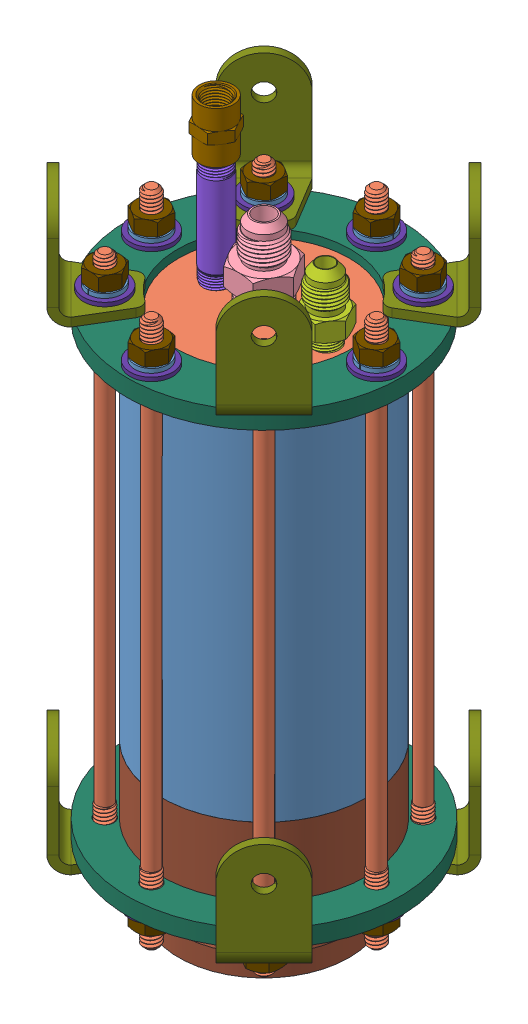
SolidWorks assembly Mojave Sphinx Thrust Chamber Assembly, configuration Default. Lengths in mm.
Overall size (101.6 253.61 101.6).
73 component instances, 20 part files, 71 mates.
Components (placement in the parent):
- CMBR-200DI-250B-525L Combustion Chamber, Mojave Sphinx-1: CMBR-200DI-250B-525L Combustion Chamber, Mojave Sphinx [Default] at origin size (76.2 133.35 76.2)
- INJC-2X8NPT-38NPT-250T20-2XO230-GENERIC Injector, Generic Orifice Pattern, Mojave Sphinx-1: INJC-2X8NPT-38NPT-250T20-2XO230-GENERIC Injector, Generic Orifice Pattern, Mojave Sphinx [Default] at (0 118.11 0) size (63.5 26.67 63.5)
- 90213A101_Inverted External Retaining Ring-1: 90213A101_Inverted External Retaining Ring [90213A101] at (0 134.3406 0) x (0 0 1) z (0 1 0) size (71.45 71.38 1.98)
- 50675K164_37 Degree Flared Fitting for Copper Tubing-1: 50675K164_37 Degree Flared Fitting for Copper Tubing [50675K164] at (0 151.003 0) x (0 1 0) z (0 0 1) size (36.97 22 19.05)
- 9368T14_High-Temperature Dry-Running 841 Bronze Sleeve Bearing-1: 9368T14_High-Temperature Dry-Running 841 Bronze Sleeve Bearing [9368T14] at (0 113.3475 0) x (1 0 0) z (0 -1 0) size (9.58 9.58 9.53)
- 90015A410_Low-Profile Ultra-Wd Truss Head Slotted Screw-1: 90015A410_Low-Profile Ultra-Wd Truss Head Slotted Screw [90015A410] at (0 108.585 0) x (-0.837169 0 -0.546944) z (0 -1 0) size (19.18 19.18 22.31)
- 50675K435_37 Degree Flared Fitting for Copper Tubing-1: 50675K435_37 Degree Flared Fitting for Copper Tubing [50675K435] at (22.86 149.485 0) x (0.90067 0 -0.434503) z (0 -1 0) size (14.2 16.4 31.34)
- 50785K171_High-Pressure Brass Pipe Nipple-1: 50785K171_High-Pressure Brass Pipe Nipple [4568K113] at (-17.78 159.385 0) x (0 1 0) z (0 0 1) size (50.88 10.57 10.53)
- 50785K91_High-Pressure Brass Pipe Fitting-1: 50785K91_High-Pressure Brass Pipe Fitting [50785K91] at (-17.78 189.23 0) x (0.837169 0 0.546944) z (0 -1 0) size (12.7 14.66 19.25)
- 9396K79_High-Temperature High-Purity Silicone O-Ring-1: 9396K79_High-Temperature High-Purity Silicone O-Ring [9396K79] at (0 129.5019 0) x (1 0 0) z (0 -1 0) size (63.65 63.65 2.62)
- 9396K79_High-Temperature High-Purity Silicone O-Ring-2: 9396K79_High-Temperature High-Purity Silicone O-Ring [9396K79] at (0 116.2431 0) x (1 0 0) z (0 -1 0) size (63.65 63.65 2.62)
- NZZL-45C20D-200E Nozzle, for Throat Insert, Mojave Sphinx-3: NZZL-45C20D-200E Nozzle, for Throat Insert, Mojave Sphinx [Default] at (0 -19.812 0) size (76.2 54.7 76.2)
- THRT-45C20D-100T Throat Insert, Spring Retained, Mojave Sphinx-1: THRT-45C20D-100T Throat Insert, Spring Retained, Mojave Sphinx [Default] at (0 -16.6021 0) size (38.1 22.41 38.1)
- 94095K114_High-Temperature Graphite Gasket - Trimmed ID-1: 94095K114_High-Temperature Graphite Gasket - Trimmed ID [94095K114] at (0 0.0318 0) x (1 0 0) z (0 1 0) size (73.03 73.03 1.59)
- 8284N57_Garter Spring-1: 8284N57_Garter Spring [8284N57] at (0 -18.5871 0) x (0.9999 0 0.014174) z (0 -1 0) size (38.9 38.9 2.59)
- FLNG-ST-25T-8X250C Flange Plate, Thrust Chamber, Mojave Sphinx-1: FLNG-ST-25T-8X250C Flange Plate, Thrust Chamber, Mojave Sphinx [Default] at (0 135.3312 0) size (101.6 6.35 101.6)
- FLNG-ST-25T-8X250C Flange Plate, Thrust Chamber, Mojave Sphinx-2: FLNG-ST-25T-8X250C Flange Plate, Thrust Chamber, Mojave Sphinx [Default] at (0 -31.75 0) size (101.6 6.35 101.6)
- BRKT-90A-125T-2X250C Bracket, Thrust Chamber Mounting, Mojave Sphinx-1: BRKT-90A-125T-2X250C Bracket, Thrust Chamber Mounting, Mojave Sphinx [Default] at (0 144.8562 0) x (0.707107 0 0.707107) z (-0.707107 0 0.707107) size (25.4 41.27 25.81)
- BRKT-90A-125T-2X250C Bracket, Thrust Chamber Mounting, Mojave Sphinx-5: BRKT-90A-125T-2X250C Bracket, Thrust Chamber Mounting, Mojave Sphinx [Default] at (0 -31.75 0) x (0.707107 0 0.707107) z (-0.707107 0 0.707107) size (25.4 41.27 25.81)
- 92141A029_18-8 Stainless Steel Washer-1: 92141A029_18-8 Stainless Steel Washer [92141A029] at (-41.91 141.6812 0) size (15.88 1.45 15.88)
- 92141A029_18-8 Stainless Steel Washer-2: 92141A029_18-8 Stainless Steel Washer [92141A029] at (-41.91 -33.1978 0) size (15.88 1.45 15.88)
- 95505A601_Medium-Strength Steel Hex Nut-2: 95505A601_Medium-Strength Steel Hex Nut [95505A601] at (-41.91 -35.9759 0) x (1 0 0) z (0 -1 0) size (11.11 12.83 6.51)
- 95505A601_Medium-Strength Steel Hex Nut-3: 95505A601_Medium-Strength Steel Hex Nut [95505A601] at (-41.91 147.4819 0) x (1 0 0) z (0 -1 0) size (11.11 12.83 6.51)
- 91102A750_Zinc-Plated Steel Split Lock Washer-1: 91102A750_Zinc-Plated Steel Split Lock Washer [91102A750] at (-41.91 143.129 0) size (12.37 1.57 12.37)
- 92141A029_18-8 Stainless Steel Washer-13: 92141A029_18-8 Stainless Steel Washer [92141A029] at (29.6348 144.8562 -29.6348) size (15.88 1.45 15.88)
- 91102A750_Zinc-Plated Steel Split Lock Washer-12: 91102A750_Zinc-Plated Steel Split Lock Washer [91102A750] at (29.6348 146.304 -29.6348) size (12.37 1.57 12.37)
- 95505A601_Medium-Strength Steel Hex Nut-14: 95505A601_Medium-Strength Steel Hex Nut [95505A601] at (29.6348 150.6569 -29.6348) x (0.867365 0 0.497673) z (0 1 0) size (11.11 12.83 6.51)
- 92141A029_18-8 Stainless Steel Washer-17: 92141A029_18-8 Stainless Steel Washer [92141A029] at (29.6348 -36.3728 -29.6348) x (0 0 -1) z (1 0 0) size (15.88 1.45 15.88)
- 95505A601_Medium-Strength Steel Hex Nut-18: 95505A601_Medium-Strength Steel Hex Nut [95505A601] at (29.6348 -39.1509 -29.6348) x (-0.837169 0 -0.546944) z (0 1 0) size (11.11 12.83 6.51)
- 90281A102_Black-Oxide Steel Setup Stud-1: 90281A102_Black-Oxide Steel Setup Stud [90281A102] at (-41.91 55.753 0) x (0 1 0) z (0 0 1) size (203.57 6.54 6.5)
- 90281A102_Black-Oxide Steel Setup Stud-5: 90281A102_Black-Oxide Steel Setup Stud [90281A102] at (29.6348 55.753 -29.6348) x (0 1 0) z (0 0 1) size (203.57 6.54 6.5)
- 92141A029_18-8 Stainless Steel Washer-3: 92141A029_18-8 Stainless Steel Washer [92141A029] at (0 -33.1978 41.91) x (0 0 -1) z (1 0 0) size (15.88 1.45 15.88)
- 92141A029_18-8 Stainless Steel Washer-4: 92141A029_18-8 Stainless Steel Washer [92141A029] at (41.91 -33.1978 0) x (-1 0 0) z (0 0 -1) size (15.88 1.45 15.88)
- 92141A029_18-8 Stainless Steel Washer-5: 92141A029_18-8 Stainless Steel Washer [92141A029] at (0 -33.1978 -41.91) x (0 0 1) z (-1 0 0) size (15.88 1.45 15.88)
- 95505A601_Medium-Strength Steel Hex Nut-4: 95505A601_Medium-Strength Steel Hex Nut [95505A601] at (0 -35.9759 41.91) x (0 0 -1) z (0 -1 0) size (11.11 12.83 6.51)
- 95505A601_Medium-Strength Steel Hex Nut-5: 95505A601_Medium-Strength Steel Hex Nut [95505A601] at (41.91 -35.9759 0) x (-1 0 0) z (0 -1 0) size (11.11 12.83 6.51)
- 95505A601_Medium-Strength Steel Hex Nut-6: 95505A601_Medium-Strength Steel Hex Nut [95505A601] at (0 -35.9759 -41.91) x (0 0 1) z (0 -1 0) size (11.11 12.83 6.51)
- 92141A029_18-8 Stainless Steel Washer-10: 92141A029_18-8 Stainless Steel Washer [92141A029] at (0 141.6812 41.91) x (0 0 -1) z (1 0 0) size (15.88 1.45 15.88)
- 92141A029_18-8 Stainless Steel Washer-11: 92141A029_18-8 Stainless Steel Washer [92141A029] at (41.91 141.6812 0) x (-1 0 0) z (0 0 -1) size (15.88 1.45 15.88)
- 92141A029_18-8 Stainless Steel Washer-12: 92141A029_18-8 Stainless Steel Washer [92141A029] at (0 141.6812 -41.91) x (0 0 1) z (-1 0 0) size (15.88 1.45 15.88)
- 95505A601_Medium-Strength Steel Hex Nut-11: 95505A601_Medium-Strength Steel Hex Nut [95505A601] at (0 147.4819 41.91) x (0 0 -1) z (0 -1 0) size (11.11 12.83 6.51)
- 95505A601_Medium-Strength Steel Hex Nut-12: 95505A601_Medium-Strength Steel Hex Nut [95505A601] at (41.91 147.4819 0) x (-1 0 0) z (0 -1 0) size (11.11 12.83 6.51)
- 95505A601_Medium-Strength Steel Hex Nut-13: 95505A601_Medium-Strength Steel Hex Nut [95505A601] at (0 147.4819 -41.91) x (0 0 1) z (0 -1 0) size (11.11 12.83 6.51)
- BRKT-90A-125T-2X250C Bracket, Thrust Chamber Mounting, Mojave Sphinx-2: BRKT-90A-125T-2X250C Bracket, Thrust Chamber Mounting, Mojave Sphinx [Default] at (0 144.8562 0) x (0.707107 0 -0.707107) z (0.707107 0 0.707107) size (25.4 41.27 25.81)
- BRKT-90A-125T-2X250C Bracket, Thrust Chamber Mounting, Mojave Sphinx-3: BRKT-90A-125T-2X250C Bracket, Thrust Chamber Mounting, Mojave Sphinx [Default] at (0 144.8562 0) x (-0.707107 0 -0.707107) z (0.707107 0 -0.707107) size (25.4 41.27 25.81)
- BRKT-90A-125T-2X250C Bracket, Thrust Chamber Mounting, Mojave Sphinx-4: BRKT-90A-125T-2X250C Bracket, Thrust Chamber Mounting, Mojave Sphinx [Default] at (0 144.8562 0) x (-0.707107 0 0.707107) z (-0.707107 0 -0.707107) size (25.4 41.27 25.81)
- 91102A750_Zinc-Plated Steel Split Lock Washer-9: 91102A750_Zinc-Plated Steel Split Lock Washer [91102A750] at (0 143.129 41.91) x (0 0 -1) z (1 0 0) size (12.37 1.57 12.37)
- 91102A750_Zinc-Plated Steel Split Lock Washer-10: 91102A750_Zinc-Plated Steel Split Lock Washer [91102A750] at (41.91 143.129 0) x (-1 0 0) z (0 0 -1) size (12.37 1.57 12.37)
- 91102A750_Zinc-Plated Steel Split Lock Washer-11: 91102A750_Zinc-Plated Steel Split Lock Washer [91102A750] at (0 143.129 -41.91) x (0 0 1) z (-1 0 0) size (12.37 1.57 12.37)
- BRKT-90A-125T-2X250C Bracket, Thrust Chamber Mounting, Mojave Sphinx-6: BRKT-90A-125T-2X250C Bracket, Thrust Chamber Mounting, Mojave Sphinx [Default] at (0 -31.75 0) x (0.707107 0 -0.707107) z (0.707107 0 0.707107) size (25.4 41.27 25.81)
- BRKT-90A-125T-2X250C Bracket, Thrust Chamber Mounting, Mojave Sphinx-7: BRKT-90A-125T-2X250C Bracket, Thrust Chamber Mounting, Mojave Sphinx [Default] at (0 -31.75 0) x (-0.707107 0 -0.707107) z (0.707107 0 -0.707107) size (25.4 41.27 25.81)
- BRKT-90A-125T-2X250C Bracket, Thrust Chamber Mounting, Mojave Sphinx-8: BRKT-90A-125T-2X250C Bracket, Thrust Chamber Mounting, Mojave Sphinx [Default] at (0 -31.75 0) x (-0.707107 0 0.707107) z (-0.707107 0 -0.707107) size (25.4 41.27 25.81)
- 92141A029_18-8 Stainless Steel Washer-18: 92141A029_18-8 Stainless Steel Washer [92141A029] at (-29.6348 -36.3728 -29.6348) x (-1 0 0) z (0 0 -1) size (15.88 1.45 15.88)
- 92141A029_18-8 Stainless Steel Washer-19: 92141A029_18-8 Stainless Steel Washer [92141A029] at (-29.6348 -36.3728 29.6348) x (0 0 1) z (-1 0 0) size (15.88 1.45 15.88)
- 92141A029_18-8 Stainless Steel Washer-20: 92141A029_18-8 Stainless Steel Washer [92141A029] at (29.6348 -36.3728 29.6348) size (15.88 1.45 15.88)
- 95505A601_Medium-Strength Steel Hex Nut-19: 95505A601_Medium-Strength Steel Hex Nut [95505A601] at (-29.6348 -39.1509 -29.6348) x (-0.546944 0 0.837169) z (0 1 0) size (11.11 12.83 6.51)
- 95505A601_Medium-Strength Steel Hex Nut-20: 95505A601_Medium-Strength Steel Hex Nut [95505A601] at (-29.6348 -39.1509 29.6348) x (0.837169 0 0.546944) z (0 1 0) size (11.11 12.83 6.51)
- 95505A601_Medium-Strength Steel Hex Nut-21: 95505A601_Medium-Strength Steel Hex Nut [95505A601] at (29.6348 -39.1509 29.6348) x (0.546944 0 -0.837169) z (0 1 0) size (11.11 12.83 6.51)
- 92141A029_18-8 Stainless Steel Washer-21: 92141A029_18-8 Stainless Steel Washer [92141A029] at (-29.6348 144.8562 -29.6348) x (0 0 -1) z (1 0 0) size (15.88 1.45 15.88)
- 92141A029_18-8 Stainless Steel Washer-22: 92141A029_18-8 Stainless Steel Washer [92141A029] at (-29.6348 144.8562 29.6348) x (-1 0 0) z (0 0 -1) size (15.88 1.45 15.88)
- 92141A029_18-8 Stainless Steel Washer-23: 92141A029_18-8 Stainless Steel Washer [92141A029] at (29.6348 144.8562 29.6348) x (0 0 1) z (-1 0 0) size (15.88 1.45 15.88)
- 91102A750_Zinc-Plated Steel Split Lock Washer-16: 91102A750_Zinc-Plated Steel Split Lock Washer [91102A750] at (-29.6348 146.304 -29.6348) x (0 0 -1) z (1 0 0) size (12.37 1.57 12.37)
- 91102A750_Zinc-Plated Steel Split Lock Washer-17: 91102A750_Zinc-Plated Steel Split Lock Washer [91102A750] at (-29.6348 146.304 29.6348) x (-1 0 0) z (0 0 -1) size (12.37 1.57 12.37)
- 91102A750_Zinc-Plated Steel Split Lock Washer-18: 91102A750_Zinc-Plated Steel Split Lock Washer [91102A750] at (29.6348 146.304 29.6348) x (0 0 1) z (-1 0 0) size (12.37 1.57 12.37)
- 95505A601_Medium-Strength Steel Hex Nut-22: 95505A601_Medium-Strength Steel Hex Nut [95505A601] at (-29.6348 150.6569 -29.6348) x (0.497673 0 -0.867365) z (0 1 0) size (11.11 12.83 6.51)
- 95505A601_Medium-Strength Steel Hex Nut-23: 95505A601_Medium-Strength Steel Hex Nut [95505A601] at (-29.6348 150.6569 29.6348) x (-0.867365 0 -0.497673) z (0 1 0) size (11.11 12.83 6.51)
- 95505A601_Medium-Strength Steel Hex Nut-24: 95505A601_Medium-Strength Steel Hex Nut [95505A601] at (29.6348 150.6569 29.6348) x (-0.497673 0 0.867365) z (0 1 0) size (11.11 12.83 6.51)
- 90281A102_Black-Oxide Steel Setup Stud-2: 90281A102_Black-Oxide Steel Setup Stud [90281A102] at (0 55.753 41.91) x (0 1 0) z (1 0 0) size (203.57 6.54 6.5)
- 90281A102_Black-Oxide Steel Setup Stud-3: 90281A102_Black-Oxide Steel Setup Stud [90281A102] at (41.91 55.753 0) x (0 1 0) z (0 0 -1) size (203.57 6.54 6.5)
- 90281A102_Black-Oxide Steel Setup Stud-4: 90281A102_Black-Oxide Steel Setup Stud [90281A102] at (0 55.753 -41.91) x (0 1 0) z (-1 0 0) size (203.57 6.54 6.5)
- 90281A102_Black-Oxide Steel Setup Stud-6: 90281A102_Black-Oxide Steel Setup Stud [90281A102] at (-29.6348 55.753 -29.6348) x (0 1 0) z (1 0 0) size (203.57 6.54 6.5)
- 90281A102_Black-Oxide Steel Setup Stud-7: 90281A102_Black-Oxide Steel Setup Stud [90281A102] at (-29.6348 55.753 29.6348) x (0 1 0) z (0 0 -1) size (203.57 6.54 6.5)
- 90281A102_Black-Oxide Steel Setup Stud-8: 90281A102_Black-Oxide Steel Setup Stud [90281A102] at (29.6348 55.753 29.6348) x (0 1 0) z (-1 0 0) size (203.57 6.54 6.5)
Mates (geometry in assembly coordinates):
- Concentric1: concentric aligned: cylinder of CMBR-200DI-250B-525L Combustion Chamber, Mojave Sphinx-1 through (0 55.7468 0) axis (0 1 0) radius 25.4; cylinder of INJC-2X8NPT-38NPT-250T20-2XO230-GENERIC Injector, Generic Orifice Pattern, Mojave Sphinx-1 through (0 144.356 0) axis (0 1 0) radius 31.75
- Concentric2: concentric aligned: cylinder of CMBR-200DI-250B-525L Combustion Chamber, Mojave Sphinx-1 through (0 55.7468 0) axis (0 1 0) radius 38.1; cylinder of NZZL-45C20D-200E Nozzle, for Throat Insert, Mojave Sphinx-3 through (0 22.128 0) axis (0 1 0) radius 38.1
- Coincident2: coincident anti-aligned: plane of CMBR-200DI-250B-525L Combustion Chamber, Mojave Sphinx-1 through (25.4 0 0) normal (0 -1 0); plane of NZZL-45C20D-200E Nozzle, for Throat Insert, Mojave Sphinx-3 through (36.5125 0 0) normal (0 1 0)
- Concentric4: concentric anti-aligned: cylinder of CMBR-200DI-250B-525L Combustion Chamber, Mojave Sphinx-1 through (0 55.7468 0) axis (0 1 0) radius 38.1; cylinder of FLNG-ST-25T-8X250C Flange Plate, Thrust Chamber, Mojave Sphinx-1 through (0 141.6812 0) axis (0 -1 0) radius 50.8
- Coincident8: coincident aligned: plane of INJC-2X8NPT-38NPT-250T20-2XO230-GENERIC Injector, Generic Orifice Pattern, Mojave Sphinx-1 through (0 118.11 0) normal (0 0 1)
- Concentric11: concentric anti-aligned: cylinder of NZZL-45C20D-200E Nozzle, for Throat Insert, Mojave Sphinx-3 through (0 22.128 0) axis (0 1 0) radius 31.75; cylinder of FLNG-ST-25T-8X250C Flange Plate, Thrust Chamber, Mojave Sphinx-2 through (0 -25.4 0) axis (0 -1 0) radius 32.258
- Coincident12: coincident anti-aligned: plane of NZZL-45C20D-200E Nozzle, for Throat Insert, Mojave Sphinx-3 through (38.1 -25.4 0) normal (0 -1 0); plane of FLNG-ST-25T-8X250C Flange Plate, Thrust Chamber, Mojave Sphinx-2 through (0 -25.4 0) normal (0 1 0)
- Concentric14: concentric aligned: cylinder of FLNG-ST-25T-8X250C Flange Plate, Thrust Chamber, Mojave Sphinx-1 through (-41.91 141.6812 0) axis (0 1 0) radius 3.3782; cylinder of 92141A029_18-8 Stainless Steel Washer-1 through (-41.91 141.6812 0) axis (0 1 0) radius 3.5687
- Concentric15: concentric aligned: cylinder of FLNG-ST-25T-8X250C Flange Plate, Thrust Chamber, Mojave Sphinx-2 through (-41.91 -25.4 0) axis (0 1 0) radius 3.3782; cylinder of 92141A029_18-8 Stainless Steel Washer-2 through (-41.91 -33.1978 0) axis (0 1 0) radius 3.5687
- Coincident16: coincident anti-aligned: plane of FLNG-ST-25T-8X250C Flange Plate, Thrust Chamber, Mojave Sphinx-2 through (0 -31.75 0) normal (0 -1 0); plane of 92141A029_18-8 Stainless Steel Washer-2 through (-41.91 -31.75 0) normal (0 1 0)
- Concentric16: concentric anti-aligned: cylinder of INJC-2X8NPT-38NPT-250T20-2XO230-GENERIC Injector, Generic Orifice Pattern, Mojave Sphinx-1 through (0 144.356 0) axis (0 1 0) radius 30.226; cylinder of 90213A101_Inverted External Retaining Ring-1 through (0 135.3312 0) axis (0 -1 0) radius 35.7251
- Coincident18: coincident anti-aligned: plane of CMBR-200DI-250B-525L Combustion Chamber, Mojave Sphinx-1 through (31.877 133.35 0) normal (0 1 0); plane of 90213A101_Inverted External Retaining Ring-1 through (0 133.35 0) normal (0 -1 0)
- Coincident19: coincident anti-aligned: plane of FLNG-ST-25T-8X250C Flange Plate, Thrust Chamber, Mojave Sphinx-1 through (0 135.3312 0) normal (0 -1 0); plane of 90213A101_Inverted External Retaining Ring-1 through (0 135.3312 0) normal (0 1 0)
- Concentric17: concentric anti-aligned: cylinder of NZZL-45C20D-200E Nozzle, for Throat Insert, Mojave Sphinx-3 through (0 22.128 0) axis (0 1 0) radius 38.1; cylinder of 94095K114_High-Temperature Graphite Gasket - Trimmed ID-1 through (0 -0.762 0) axis (0 -1 0) radius 36.5125
- Coincident20: coincident anti-aligned: plane of NZZL-45C20D-200E Nozzle, for Throat Insert, Mojave Sphinx-3 through (36.5125 -0.762 0) normal (0 1 0); plane of 94095K114_High-Temperature Graphite Gasket - Trimmed ID-1 through (0 -0.762 -32.262) normal (0 -1 0)
- Coincident21: coincident anti-aligned: plane of 92141A029_18-8 Stainless Steel Washer-2 through (-41.91 -33.1978 0) normal (0 -1 0); plane of 95505A601_Medium-Strength Steel Hex Nut-2 through (-47.4663 -33.1978 3.2079) normal (0 1 0)
- Concentric20: concentric aligned: cylinder of 92141A029_18-8 Stainless Steel Washer-2 through (-41.91 -31.75 0) axis (0 -1 0) radius 7.9375; circle of 95505A601_Medium-Strength Steel Hex Nut-2
- Concentric23: concentric anti-aligned: circle of 92141A029_18-8 Stainless Steel Washer-1; circle of 95505A601_Medium-Strength Steel Hex Nut-3
- Coincident27: coincident anti-aligned: plane of FLNG-ST-25T-8X250C Flange Plate, Thrust Chamber, Mojave Sphinx-1 through (0 141.6812 0) normal (0 1 0); plane of BRKT-90A-125T-2X250C Bracket, Thrust Chamber Mounting, Mojave Sphinx-1 through (0 141.6812 0) normal (0 -1 0)
- Concentric29: concentric aligned: cylinder of FLNG-ST-25T-8X250C Flange Plate, Thrust Chamber, Mojave Sphinx-1 through (29.6348 141.6812 -29.6348) axis (0 1 0) radius 3.3782; cylinder of BRKT-90A-125T-2X250C Bracket, Thrust Chamber Mounting, Mojave Sphinx-1 through (29.6348 141.6812 -29.6348) axis (0 1 0) radius 3.3909
- Angle1: planar angle = 2.356194 rad aligned: plane of BRKT-90A-125T-2X250C Bracket, Thrust Chamber Mounting, Mojave Sphinx-1 through (40.4112 144.8562 -40.4112) normal (0.707107 0 -0.707107)
- Concentric30: concentric aligned: cylinder of 92141A029_18-8 Stainless Steel Washer-1 through (-41.91 143.129 0) axis (0 -1 0) radius 7.9375; cylinder of 91102A750_Zinc-Plated Steel Split Lock Washer (1)-1 through (-41.91 144.7038 0) axis (0 -1 0) radius 6.1849
- Coincident30: coincident anti-aligned: plane of 92141A029_18-8 Stainless Steel Washer-1 through (-41.91 143.129 0) normal (0 1 0); plane of 91102A750_Zinc-Plated Steel Split Lock Washer (1)-1 through (-41.91 143.129 0) normal (0 -1 0)
- Coincident31: coincident anti-aligned: plane of 95505A601_Medium-Strength Steel Hex Nut-3 through (-47.4663 144.7038 3.2079) normal (0 -1 0); plane of 91102A750_Zinc-Plated Steel Split Lock Washer (1)-1 through (-41.91 144.7038 0) normal (0 1 0)
- Coincident33: coincident anti-aligned: plane of BRKT-90A-125T-2X250C Bracket, Thrust Chamber Mounting, Mojave Sphinx-3 through (0 144.8562 0) normal (0 1 0); plane of 92141A029_18-8 Stainless Steel Washer-13 through (29.6348 144.8562 -29.6348) normal (0 -1 0)
- Coincident34: coincident anti-aligned: plane of 92141A029_18-8 Stainless Steel Washer-13 through (29.6348 146.304 -29.6348) normal (0 1 0); plane of 91102A750_Zinc-Plated Steel Split Lock Washer (1)-12 through (29.6348 146.304 -29.6348) normal (0 -1 0)
- Concentric33: concentric aligned: cylinder of 92141A029_18-8 Stainless Steel Washer-13 through (29.6348 146.304 -29.6348) axis (0 -1 0) radius 7.9375; cylinder of 91102A750_Zinc-Plated Steel Split Lock Washer (1)-12 through (29.6348 147.8788 -29.6348) axis (0 -1 0) radius 6.1849
- Coincident35: coincident anti-aligned: plane of 91102A750_Zinc-Plated Steel Split Lock Washer (1)-12 through (29.6348 147.8788 -29.6348) normal (0 1 0); plane of 95505A601_Medium-Strength Steel Hex Nut-14 through (26.412 147.8788 -35.1825) normal (0 -1 0)
- Concentric34: concentric anti-aligned: cylinder of 91102A750_Zinc-Plated Steel Split Lock Washer (1)-12 through (29.6348 147.8788 -29.6348) axis (0 -1 0) radius 6.1849; circle of 95505A601_Medium-Strength Steel Hex Nut-14
- Coincident36: coincident anti-aligned: plane of FLNG-ST-25T-8X250C Flange Plate, Thrust Chamber, Mojave Sphinx-2 through (0 -31.75 0) normal (0 -1 0); plane of BRKT-90A-125T-2X250C Bracket, Thrust Chamber Mounting, Mojave Sphinx-5 through (0 -31.75 0) normal (0 1 0)
- Concentric37: concentric aligned: cylinder of BRKT-90A-125T-2X250C Bracket, Thrust Chamber Mounting, Mojave Sphinx-5 through (29.6348 -34.925 -29.6348) axis (0 1 0) radius 3.3909; cylinder of 92141A029_18-8 Stainless Steel Washer-17 through (29.6348 -36.3728 -29.6348) axis (0 1 0) radius 3.5687
- Coincident37: coincident anti-aligned: plane of BRKT-90A-125T-2X250C Bracket, Thrust Chamber Mounting, Mojave Sphinx-5 through (0 -34.925 0) normal (0 -1 0); plane of 92141A029_18-8 Stainless Steel Washer-17 through (29.6348 -34.925 -29.6348) normal (0 1 0)
- Coincident38: coincident anti-aligned: plane of 92141A029_18-8 Stainless Steel Washer-17 through (29.6348 -36.3728 -29.6348) normal (0 -1 0); plane of 95505A601_Medium-Strength Steel Hex Nut-18 through (32.5318 -36.3728 -23.9103) normal (0 1 0)
- Coincident39: coincident anti-aligned: plane of FLNG-ST-25T-8X250C Flange Plate, Thrust Chamber, Mojave Sphinx-1 through (0 141.6812 0) normal (0 1 0); plane of 92141A029_18-8 Stainless Steel Washer-10 through (0 141.6812 41.91) normal (0 -1 0)
- Concentric39: concentric anti-aligned: cylinder of BRKT-90A-125T-2X250C Bracket, Thrust Chamber Mounting, Mojave Sphinx-1 through (29.6348 141.6812 -29.6348) axis (0 1 0) radius 3.3909; cylinder of 92141A029_18-8 Stainless Steel Washer-13 through (29.6348 146.304 -29.6348) axis (0 -1 0) radius 7.9375
- Concentric41: concentric aligned: cylinder of FLNG-ST-25T-8X250C Flange Plate, Thrust Chamber, Mojave Sphinx-2 through (29.6348 -25.4 -29.6348) axis (0 1 0) radius 3.3782; cylinder of BRKT-90A-125T-2X250C Bracket, Thrust Chamber Mounting, Mojave Sphinx-5 through (29.6348 -34.925 -29.6348) axis (0 1 0) radius 3.3909
- Concentric42: concentric anti-aligned: cylinder of FLNG-ST-25T-8X250C Flange Plate, Thrust Chamber, Mojave Sphinx-2 through (0 -25.4 0) axis (0 -1 0) radius 50.8; cylinder of BRKT-90A-125T-2X250C Bracket, Thrust Chamber Mounting, Mojave Sphinx-5 through (0 -34.925 0) axis (0 1 0) radius 31.75
- Concentric43: concentric anti-aligned: circle of 92141A029_18-8 Stainless Steel Washer-17; circle of 95505A601_Medium-Strength Steel Hex Nut-18
- Concentric44: concentric anti-aligned: cylinder of FLNG-ST-25T-8X250C Flange Plate, Thrust Chamber, Mojave Sphinx-1 through (-41.91 141.6812 0) axis (0 1 0) radius 3.3782; cylinder of 90281A102_Black-Oxide Steel Setup Stud-1 through (-41.91 -45.847 0) axis (0 -1 0) radius 2.8575
- Width2: width anti-aligned: plane of 90281A102_Black-Oxide Steel Setup Stud-1 through (-41.91 -45.847 0) normal (0 -1 0); plane of 90281A102_Black-Oxide Steel Setup Stud-1 through (-43.815 157.353 0) normal (0 1 0); plane of 95505A601_Medium-Strength Steel Hex Nut-3 through (-47.4663 150.2601 3.2079) normal (0 1 0); plane of 95505A601_Medium-Strength Steel Hex Nut-2 through (-47.4663 -38.754 3.2079) normal (0 -1 0)
- Concentric45: concentric anti-aligned: cylinder of FLNG-ST-25T-8X250C Flange Plate, Thrust Chamber, Mojave Sphinx-1 through (29.6348 141.6812 -29.6348) axis (0 1 0) radius 3.3782; cylinder of 90281A102_Black-Oxide Steel Setup Stud-5 through (29.6348 -45.847 -29.6348) axis (0 -1 0) radius 2.8575
- Width3: width anti-aligned: plane of 90281A102_Black-Oxide Steel Setup Stud-5 through (29.6348 -45.847 -29.6348) normal (0 -1 0); plane of 90281A102_Black-Oxide Steel Setup Stud-5 through (27.7298 157.353 -29.6348) normal (0 1 0); plane of 95505A601_Medium-Strength Steel Hex Nut-14 through (26.412 153.435 -35.1825) normal (0 1 0); plane of 95505A601_Medium-Strength Steel Hex Nut-18 through (32.5318 -41.9291 -23.9103) normal (0 -1 0)
- Coincident43: coincident anti-aligned: plane of INJC-2X8NPT-38NPT-250T20-2XO230-GENERIC Injector, Generic Orifice Pattern, Mojave Sphinx-1 through (-31.75 133.35 0) normal (0 1 0); plane of 90213A101_Inverted External Retaining Ring-1 through (0 133.35 0) normal (0 -1 0)
- Concentric50: concentric anti-aligned: cylinder of INJC-2X8NPT-38NPT-250T20-2XO230-GENERIC Injector, Generic Orifice Pattern, Mojave Sphinx-1 through (0 139.065 0) axis (0 1 0) radius 7.1374; cylinder of 50675K164_37 Degree Flared Fitting for Copper Tubing-1 through (0 146.939 0) axis (0 -1 0) radius 3.81
- Distance8: distance = 6.35 mm anti-aligned: plane of 50675K164_37 Degree Flared Fitting for Copper Tubing-1 through (0 132.715 0) normal (0 -1 0); plane of INJC-2X8NPT-38NPT-250T20-2XO230-GENERIC Injector, Generic Orifice Pattern, Mojave Sphinx-1 through (-31.75 139.065 0) normal (0 1 0)
- Concentric56: concentric anti-aligned: cylinder of INJC-2X8NPT-38NPT-250T20-2XO230-GENERIC Injector, Generic Orifice Pattern, Mojave Sphinx-1 through (0 118.11 0) axis (0 -1 0) radius 2.5527; cylinder of 9368T14_High-Temperature Dry-Running 841 Bronze Sleeve Bearing-1 through (0 108.585 0) axis (0 1 0) radius 3.1877
- Coincident49: coincident anti-aligned: plane of INJC-2X8NPT-38NPT-250T20-2XO230-GENERIC Injector, Generic Orifice Pattern, Mojave Sphinx-1 through (-25.4 118.11 0) normal (0 -1 0); plane of 9368T14_High-Temperature Dry-Running 841 Bronze Sleeve Bearing-1 through (0 118.11 0) normal (0 1 0)
- Concentric59: concentric aligned: cylinder of 9368T14_High-Temperature Dry-Running 841 Bronze Sleeve Bearing-1 through (0 108.585 0) axis (0 1 0) radius 3.1877; circle of 90015A410_Low-Profile Ultra-Wd Truss Head Slotted Screw-1
- Coincident51: coincident anti-aligned: plane of 9368T14_High-Temperature Dry-Running 841 Bronze Sleeve Bearing-1 through (0 108.585 0) normal (0 -1 0); plane of 90015A410_Low-Profile Ultra-Wd Truss Head Slotted Screw-1 through (8.0272 108.585 5.2444) normal (0 1 0)
- Coincident52: coincident anti-aligned: plane of NZZL-45C20D-200E Nozzle, for Throat Insert, Mojave Sphinx-3 through (19.2405 -30.245 0) normal (0 1 0); plane of THRT-45C20D-100T Throat Insert, Spring Retained, Mojave Sphinx-1 through (19.05 -30.245 0) normal (0 -1 0)
- Concentric62: concentric anti-aligned: cylinder of NZZL-45C20D-200E Nozzle, for Throat Insert, Mojave Sphinx-3 through (0 22.128 0) axis (0 1 0) radius 19.7485; circle of 8284N57_Garter Spring-1
- Concentric63: concentric aligned: cylinder of NZZL-45C20D-200E Nozzle, for Throat Insert, Mojave Sphinx-3 through (0 22.128 0) axis (0 1 0) radius 19.2405; cylinder of THRT-45C20D-100T Throat Insert, Spring Retained, Mojave Sphinx-1 through (0 28.177 0) axis (0 1 0) radius 19.05
- Tangent1: tangent: plane of ? through (19.05 -19.812 0) normal (0 1 0); face of ?
- Concentric64: concentric anti-aligned: cylinder of INJC-2X8NPT-38NPT-250T20-2XO230-GENERIC Injector, Generic Orifice Pattern, Mojave Sphinx-1 through (22.86 139.065 0) axis (0 1 0) radius 4.2164; cylinder of 50675K435_37 Degree Flared Fitting for Copper Tubing-1 through (22.86 133.985 0) axis (0 -1 0) radius 3
- Distance10: distance = 5.08 mm anti-aligned: plane of 50675K435_37 Degree Flared Fitting for Copper Tubing-1 through (24.1635 133.985 2.702) normal (0 -1 0); plane of INJC-2X8NPT-38NPT-250T20-2XO230-GENERIC Injector, Generic Orifice Pattern, Mojave Sphinx-1 through (-31.75 139.065 0) normal (0 1 0)
- Coincident53: coincident aligned: plane of CMBR-200DI-250B-525L Combustion Chamber, Mojave Sphinx-1 through (0 0 0) normal (0 0 1)
- Coincident54: coincident aligned: plane of CMBR-200DI-250B-525L Combustion Chamber, Mojave Sphinx-1 through (0 0 0) normal (0 1 0)
- Coincident55: coincident aligned: plane of CMBR-200DI-250B-525L Combustion Chamber, Mojave Sphinx-1 through (0 0 0) normal (1 0 0)
- Concentric65: concentric anti-aligned: circle of INJC-2X8NPT-38NPT-250T20-2XO230-BASIC Injector, Basic Orifice Pattern, Mojave Sphinx-1; cylinder of 50785K171_High-Pressure Brass Pipe Nipple-1 through (-17.78 144.4223 0) axis (0 -1 0) radius 5.1435
- Distance11: distance = 5.08 mm anti-aligned: plane of 50785K171_High-Pressure Brass Pipe Nipple-1 through (-17.78 133.985 0) normal (0 -1 0); plane of INJC-2X8NPT-38NPT-250T20-2XO230-GENERIC Injector, Generic Orifice Pattern, Mojave Sphinx-1 through (-31.75 139.065 0) normal (0 1 0)
- Concentric66: concentric aligned: cylinder of 50785K171_High-Pressure Brass Pipe Nipple-1 through (-17.78 144.4223 0) axis (0 -1 0) radius 5.1435; cylinder of 50785K91_High-Pressure Brass Pipe Fitting (2)-1 through (-17.78 179.705 0) axis (0 -1 0) radius 6.35
- Distance12: distance = 5.08 mm anti-aligned: plane of 50785K91_High-Pressure Brass Pipe Fitting (2)-1 through (-17.78 179.705 0) normal (0 -1 0); plane of 50785K171_High-Pressure Brass Pipe Nipple-1 through (-17.78 184.785 0) normal (0 1 0)
- Parallel1: parallel anti-aligned: plane of 9396K79_High-Temperature High-Purity Silicone O-Ring-1 through (0 129.5019 0) normal (0 -1 0)
- Coincident57: coincident aligned: plane of 9396K79_High-Temperature High-Purity Silicone O-Ring-1 through (0 129.5019 0) normal (1 0 0)
- Coincident58: coincident aligned: plane of 9396K79_High-Temperature High-Purity Silicone O-Ring-1 through (0 129.5019 0) normal (0 0 1)
- Parallel2: parallel anti-aligned: plane of 9396K79_High-Temperature High-Purity Silicone O-Ring-2 through (0 116.2431 0) normal (0 -1 0)
- Coincident60: coincident aligned: plane of 9396K79_High-Temperature High-Purity Silicone O-Ring-2 through (0 116.2431 0) normal (0 0 1)
- Coincident61: coincident aligned: plane of 9396K79_High-Temperature High-Purity Silicone O-Ring-2 through (0 116.2431 0) normal (1 0 0)
- Distance13: distance = 1.3081 mm aligned: plane of 9396K79_High-Temperature High-Purity Silicone O-Ring-1 through (0 129.5019 0) normal (0 -1 0); plane of INJC-2X8NPT-38NPT-250T20-2XO230-GENERIC Injector, Generic Orifice Pattern, Mojave Sphinx-1 through (-31.75 130.81 0) normal (0 -1 0)
- Tangent2: tangent anti-aligned: plane of INJC-2X8NPT-38NPT-250T20-2XO230-GENERIC Injector, Generic Orifice Pattern, Mojave Sphinx-1 through (-29.591 114.935 0) normal (0 1 0); torus of 9396K79_High-Temperature High-Purity Silicone O-Ring-2
- Tangent3: tangent anti-aligned: plane of THRT-45C20D-100T Throat Insert, Spring Retained, Mojave Sphinx-1 through (19.05 -19.7771 0) normal (0 1 0); edge_curve of 8284N57_Garter Spring-1
